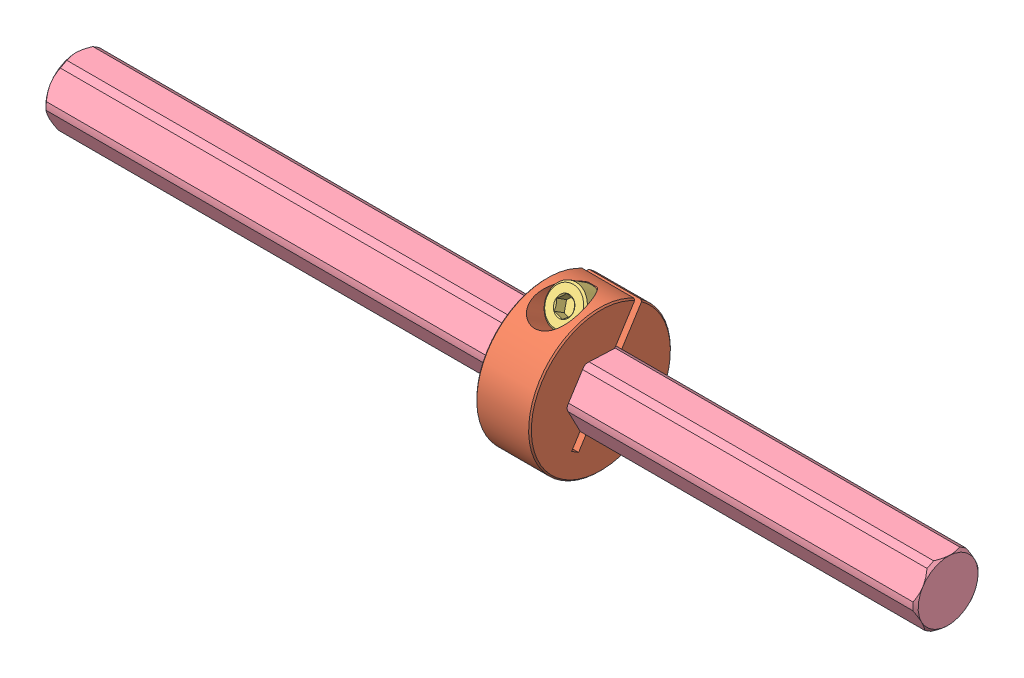
SolidWorks assembly BL Wheel, configuration Default. Lengths in mm.
Overall size (160 36.65 36.37).
5 component instances, 4 part files, 3 mates.
Components (placement in the parent):
- 12mm ID 1mm Thick Shim.step-1: 12mm ID 1mm Thick Shim.step [Default] at (74.862 410.9212 381.6675) x (0 -0.173258 -0.984876) z (0 0.984876 -0.173258) size (15 1 15)
- 12mm Axle Collar.STEP-1: 12mm Axle Collar.STEP [Default] at (61.3108 398.0183 360.6125) x (0 -0.536778 -0.843724) z (0 -0.843724 0.536778) size (26 10 26.9)
  - 2910-1026-4012.STEP-1: 2910-1026-4012.STEP [Default] at (-24.6906 18.5512 0.4154) size (26 10 25.98)
  - 2800-0004-0012_90128A207.STEP-1: 2800-0004-0012_90128A207.STEP [Default] at (-16.4406 18.5512 -8.5319) x (0 0.713618 0.700535) z (1 0 0) size (7 7 16.01)
- 12mm REX 160mm-1: 12mm REX 160mm [Default] at (68.562 410.9212 381.6675) x (0 -0.886725 -0.462297) z (0 -0.462297 0.886725) size (12 160 12.01)
Mates (geometry in assembly coordinates):
- Coincident2: coincident: plane of 12mm Axle Collar.STEP-1/2910-1026-4012.STEP-1 through (70.0402 408.3786 386.5445) normal (0 0.462297 -0.886725); plane of 12mm REX 160mm-1 through (148.562 408.3786 386.5445) normal (0 -0.462297 0.886725)
- Coincident3: coincident: plane of 12mm ID 1mm Thick Shim.step-1 through (74.862 410.9212 381.6675) normal (1 0 0); plane of 12mm Axle Collar.STEP-1/2910-1026-4012.STEP-1 through (74.862 410.9212 381.6675) normal (-1 0 0)
- Coincident4: coincident: plane of 12mm Axle Collar.STEP-1/2910-1026-4012.STEP-1 through (70.0402 407.9689 377.027) normal (0 0.536778 0.843724); plane of 12mm REX 160mm-1 through (148.562 407.9689 377.027) normal (0 -0.536778 -0.843724)
